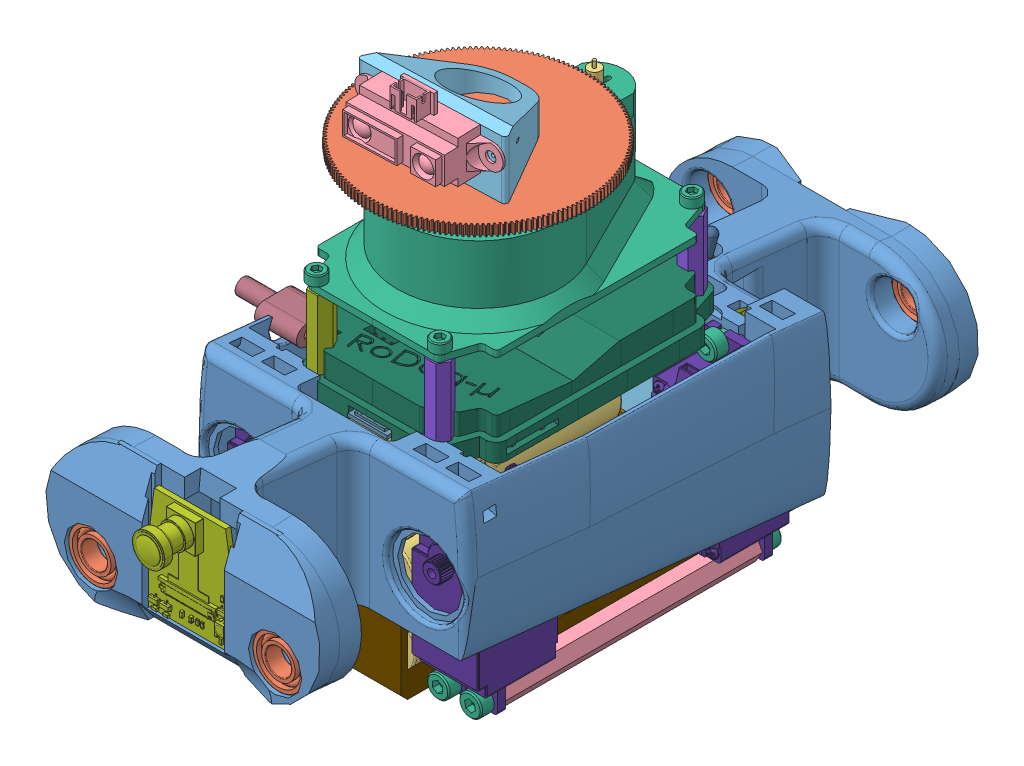
SolidWorks assembly body, configuration Default. Lengths in mm.
Overall size (109.19 147.84 215.45).
83 component instances, 28 part files, 130 mates.
Components (placement in the parent):
- Chasis-1: Chasis [Default] at (0 30 0) x (-1 0 0) z (0 0 1) size (106.67 62.56 205.11)
- radial ball bearing_68_am-1: radial ball bearing_68_am [AFBMA 20.1 - 28-8 - 12,SI,NC,12_68] at (28.5 0 98.3749) x (0 0 -1) z (1 0 0) size (5 16 16)
- radial ball bearing_68_am-2: radial ball bearing_68_am [AFBMA 20.1 - 28-8 - 12,SI,NC,12_68] at (-28.5 0 98.3749) x (0 0 -1) z (1 0 0) size (5 16 16)
- radial ball bearing_68_am-3: radial ball bearing_68_am [AFBMA 20.1 - 28-8 - 12,SI,NC,12_68] at (28.5 0 -98.3749) x (0 0 1) z (-0.94079 -0.338989 0) size (5 16 16)
- radial ball bearing_68_am-4: radial ball bearing_68_am [AFBMA 20.1 - 28-8 - 12,SI,NC,12_68] at (-28.5 0 -98.3749) x (0 0 1) z (-1 0 0) size (5 16 16)
- batteries-1: batteries [Default] at (0 -2.9 15.9266) x (0 -1 0) z (0 0 1) size (60.35 42.06 66)
  - 18650Model-std-11: 18650Model-std [Default] at (-9 -9 -32) x (1 0 0) z (0 0 -1) size (18 18 65)
  - 18650Model-std-12: 18650Model-std [Default] at (9 -9 32) x (-0.155006 -0.987914 0) z (0 0 1) size (18 18 65)
  - 18650Model-std-13: 18650Model-std [Default] at (-9 9 -32) x (0.41216 -0.911111 0) z (0 0 -1) size (18 18 65)
  - 18650Model-std-14: 18650Model-std [Default] at (9 9 32) x (0.93408 -0.357065 0) z (0 0 1) size (18 18 65)
  - 18650Model-std-15: 18650Model-std [Default] at (27 -9 32) x (-0.934528 0.355889 0) z (0 0 1) size (18 18 65)
  - 18650Model-std-16: 18650Model-std [Default] at (27 9 32) x (0.84116 -0.540786 0) z (0 0 1) size (18 18 65)
- 80x4mm standoff-1: 80x4mm standoff [Default] at (33.5 -36.4 -39.9266) x (0.999176 -0.040598 0) z (0 0 1) size (8.08 7 80)
- 80x4mm standoff-2: 80x4mm standoff [Default] at (-33.5 -36.4 -39.9266) x (0.828718 -0.559667 0) z (0 0 1) size (8.08 7 80)
- 1X08-BIG.step-1: 1X08-BIG.step [Default] at (0 -27.0348 -47.5734) x (0 0 -1) z (0 -1 0) size (10 31 29.5)
- socket head cap screw_am-1: socket head cap screw_am [B18.3.1M - 4 x 0.7 x 10 Hex SHCS -- 10NHX] at (-33.5 -36.4 46.5734) x (0 0 -1) z (1 0 0) size (14 7 7)
- socket head cap screw_am-2: socket head cap screw_am [B18.3.1M - 4 x 0.7 x 10 Hex SHCS -- 10NHX] at (-23.5 -36.4 46.5734) x (0 0 -1) z (0.464802 -0.885415 0) size (14 7 7)
- socket head cap screw_am-3: socket head cap screw_am [B18.3.1M - 4 x 0.7 x 10 Hex SHCS -- 10NHX] at (23.5 -36.4 46.5734) x (0 0 -1) z (1 0 0) size (14 7 7)
- socket head cap screw_am-4: socket head cap screw_am [B18.3.1M - 4 x 0.7 x 10 Hex SHCS -- 10NHX] at (33.5 -36.4 46.5734) x (0 0 -1) z (0.972971 0.230929 0) size (14 7 7)
- socket head cap screw_am-5: socket head cap screw_am [B18.3.1M - 4 x 0.7 x 10 Hex SHCS -- 10NHX] at (33.5 -36.4 -46.5734) x (0 0 1) z (-1 0 0) size (14 7 7)
- socket head cap screw_am-6: socket head cap screw_am [B18.3.1M - 4 x 0.7 x 10 Hex SHCS -- 10NHX] at (23.5 -36.4 -46.5734) x (0 0 1) z (-1 0 0) size (14 7 7)
- socket head cap screw_am-7: socket head cap screw_am [B18.3.1M - 4 x 0.7 x 10 Hex SHCS -- 10NHX] at (-33.5 -36.4 -46.5734) x (0 0 1) z (-1 0 0) size (14 7 7)
- socket head cap screw_am-8: socket head cap screw_am [B18.3.1M - 4 x 0.7 x 10 Hex SHCS -- 10NHX] at (-23.5 -36.4 -46.5734) x (0 0 1) z (-1 0 0) size (14 7 7)
- socket head cap screw_am-13: socket head cap screw_am [B18.3.1M - 4 x 0.7 x 10 Hex SHCS -- 10NHX] at (-33.5 13 36.0734) x (0 0 1) z (-0.497518 -0.867454 0) size (14 7 7)
- socket head cap screw_am-14: socket head cap screw_am [B18.3.1M - 4 x 0.7 x 10 Hex SHCS -- 10NHX] at (-23.5 13 36.0734) x (0 0 1) z (-0.937162 -0.348893 0) size (14 7 7)
- socket head cap screw_am-15: socket head cap screw_am [B18.3.1M - 4 x 0.7 x 10 Hex SHCS -- 10NHX] at (23.5 13 -36.0734) x (0 0 -1) z (0.999531 -0.030613 0) size (14 7 7)
- socket head cap screw_am-16: socket head cap screw_am [B18.3.1M - 4 x 0.7 x 10 Hex SHCS -- 10NHX] at (33.5 13 -36.0734) x (0 0 -1) z (0.970522 0.241011 0) size (14 7 7)
- socket head cap screw_am-17: socket head cap screw_am [B18.3.1M - 4 x 0.7 x 10 Hex SHCS -- 10NHX] at (23.5 13 36.0734) x (0 0 1) z (-0.883708 -0.468039 0) size (14 7 7)
- socket head cap screw_am-18: socket head cap screw_am [B18.3.1M - 4 x 0.7 x 10 Hex SHCS -- 10NHX] at (33.5 13 36.0734) x (0 0 1) z (-0.911074 -0.412244 0) size (14 7 7)
- socket head cap screw_am-19: socket head cap screw_am [B18.3.1M - 4 x 0.7 x 10 Hex SHCS -- 10NHX] at (-33.5 13 -36.0734) x (0 0 -1) z (0.998285 -0.058546 0) size (14 7 7)
- socket head cap screw_am-20: socket head cap screw_am [B18.3.1M - 4 x 0.7 x 10 Hex SHCS -- 10NHX] at (-23.5 13 -36.0734) x (0 0 -1) z (0.993249 -0.115998 0) size (14 7 7)
- mobo2_camSLDPRT-1: mobo2_camSLDPRT [Default] at (-51.3967 -126.1208 97.875) x (0 1 0) z (0 0 1) size (33.03 26.96 15.7)
- FUJISOKU ATE 2D.stp-1: FUJISOKU ATE 2D.stp [Default] at (0.3584 5.2835 -67.8989) x (0 0 -1) z (0 1 0) size (9.5 5 23.29)
  - SW7.stp-1: SW7.stp [Default] at (-7.8256 0.3584 -3.9) size (9.5 5 7.8)
  - SW8.stp-1: SW8.stp [Default] at (-7.8256 0.3584 4.4) x (1 0 0) z (0 0 -1) size (9.5 5 10)
  - SW3.stp-1: SW3.stp [Default] at (-7.8256 0.3584 7.4) x (0.978148 0 -0.207912) z (0 -1 0) size (3.5 10.25 3.8)
  - SW10.stp-1: SW10.stp [Default] at (-7.8256 1.6284 -3.4) x (1 0 0) z (0 1 0) size (1 3.81 0.59)
  - SW10.stp-2: SW10.stp [Default] at (-5.2856 1.6284 -3.4) x (1 0 0) z (0 1 0) size (1 3.81 0.59)
  - SW10.stp-3: SW10.stp [Default] at (-10.3656 1.6284 -3.4) x (1 0 0) z (0 1 0) size (1 3.81 0.59)
  - SW10_MIR.stp-1: SW10_MIR.stp [Default] at (-10.3656 -0.9116 -3.4) x (1 0 0) z (0 1 0) size (1 3.81 0.59)
  - SW10_MIR.stp-2: SW10_MIR.stp [Default] at (-5.2856 -0.9116 -3.4) x (1 0 0) z (0 1 0) size (1 3.81 0.59)
  - SW10_MIR.stp-3: SW10_MIR.stp [Default] at (-7.8256 -0.9116 -3.4) x (1 0 0) z (0 1 0) size (1 3.81 0.59)
- USB C mockup-1: USB C mockup [Default] at (-25.8477 21.8173 27.4357) x (0.000257 0 1) z (-1 0 0.000257) size (13 6 30)
- RodogMobo-1: RodogMobo [Default] at (-18.2824 20.1 -37.4091) x (0.000772 0 1) z (0 1 0) size (86.12 60.15 16.5)
- Mobo cover-1: Mobo cover [Default] at (0 19.7 0) x (1 0 0) z (0 1 0) size (60.01 87.25 12.67)
- socket head cap screw_am-21: socket head cap screw_am [B18.3.1M - 3 x 0.5 x 10 Hex SHCS -- 10NHX] at (-18.2187 28.7 40.7111) x (0 -1 0) z (0 0 1) size (13 5.5 5.5) (hidden)
- socket head cap screw_am-22: socket head cap screw_am [B18.3.1M - 3 x 0.5 x 10 Hex SHCS -- 10NHX] at (-18.279 28.7 -37.3889) x (0 -1 0) z (-0.207293 0 -0.978279) size (13 5.5 5.5) (hidden)
- socket head cap screw_am-23: socket head cap screw_am [B18.3.1M - 3 x 0.5 x 10 Hex SHCS -- 10NHX] at (18.221 28.7 -37.4171) x (0 -1 0) z (0 0 1) size (13 5.5 5.5) (hidden)
- socket head cap screw_am-24: socket head cap screw_am [B18.3.1M - 3 x 0.5 x 10 Hex SHCS -- 10NHX] at (18.2813 28.7 40.6829) x (0 -1 0) z (0 0 1) size (13 5.5 5.5) (hidden)
- hex nut style 1_am-2: hex nut style 1_am [B18.2.4.1M - Hex nut, Style 1,  M4 x 0.7 --D-N] at (-33.5 13 50.1734) x (-0.244529 0.969642 0) z (0 0 1) size (7 8.08 3.2)
- hex nut style 1_am-3: hex nut style 1_am [B18.2.4.1M - Hex nut, Style 1,  M4 x 0.7 --D-N] at (-23.5 13 50.1734) x (0.692093 0.721808 0) z (0 0 1) size (7 8.08 3.2)
- hex nut style 1_am-4: hex nut style 1_am [B18.2.4.1M - Hex nut, Style 1,  M4 x 0.7 --D-N] at (33.5 13 46.9734) x (-0.965845 0.259119 0) z (0 0 -1) size (7 8.08 3.2)
- hex nut style 1_am-5: hex nut style 1_am [B18.2.4.1M - Hex nut, Style 1,  M4 x 0.7 --D-N] at (23.5 13 46.9734) x (0.793594 0.608447 0) z (0 0 -1) size (7 8.08 3.2)
- hex nut style 1_am-6: hex nut style 1_am [B18.2.4.1M - Hex nut, Style 1,  M4 x 0.7 --D-N] at (-23.5 13 -50.1734) x (-0.5 0.866025 0) z (0 0 -1) size (7 8.08 3.2)
- hex nut style 1_am-7: hex nut style 1_am [B18.2.4.1M - Hex nut, Style 1,  M4 x 0.7 --D-N] at (23.5 13 -46.9734) x (-1 0 0) z (0 0 1) size (7 8.08 3.2)
- hex nut style 1_am-8: hex nut style 1_am [B18.2.4.1M - Hex nut, Style 1,  M4 x 0.7 --D-N] at (-33.5 13 -46.9734) x (-0.793594 0.608447 0) z (0 0 1) size (7 8.08 3.2)
- hex nut style 1_am-9: hex nut style 1_am [B18.2.4.1M - Hex nut, Style 1,  M4 x 0.7 --D-N] at (33.5 13 -46.9734) x (-0.254777 -0.967 0) z (0 0 1) size (7 8.08 3.2)
- HS-8775MG-1: HS-8775MG [Default] at (-38.5 8 24.0734) x (0 -1 0) z (-1 0 0) size (54.4 29.4 21)
- HS-8775MG-2: HS-8775MG [Default] at (-18.5 8 -24.0734) x (0 -1 0) z (1 0 0) size (54.4 29.4 21)
- HS-8775MG-3: HS-8775MG [Default] at (38.5 8 -24.0734) x (0 -1 0) z (1 0 0) size (54.4 29.4 21)
- HS-8775MG-4: HS-8775MG [Default] at (18.5 8 24.0734) x (0 -1 0) z (-1 0 0) size (54.4 29.4 21)
- Battery mount-1: Battery mount [Default] at (-38.5 8 40.0734) x (0 1 0) z (0 0 -1) size (23.66 55.5 105.15)
- 2D scanner assembly-1: 2D scanner assembly [Default] at (0.0023 52 10.5725) x (0 0 -1) z (1 0 0) size (85.67 58.5 70.17)
  - Slip Ring-1: Slip Ring [Default] at origin size (44 35.4 44)
  - spur gear_am-3: spur gear_am [Metric - Spur gear 0.4M 168T 20PA 3FW ---S168O19H8L12N] at (0 29.5 0) x (0 -1 0) z (0.999472 0 -0.032496) size (8 67.99 67.99)
  - DC Motor-1: DC Motor [Default] at (36 7 0) x (1 0 0) z (0 1 0) size (12.1 10 25)
  - 2Y0A21-1: 2Y0A21 [Default] at (-14.9921 41.0001 0.4874) x (-0.032496 0 -0.999472) z (-0.999472 0 0.032496) size (44.5 19 13.5)
  - Part7^2D scanner assembly-1: Part7^2D scanner assembly [Default] at (0 29.5 0) x (0.999472 0 -0.032496) z (0 1 0) size (28 44.18 18) (virtual)
  - Part8^2D scanner assembly-1: Part8^2D scanner assembly [Default] at (0 19.1 0) x (-1 0 0) z (0 -1 0) size (83.25 58.72 30) (virtual)
  - RodogMobo-1: RodogMobo [Default] at (-30.1305 -16.6 18.2824) x (1 0 -0.000772) z (0 1 0) size (86.12 60.15 16.5) (hidden)
  - socket head cap screw_am-1: socket head cap screw_am [B18.3.1M - 3 x 0.5 x 25 Hex SHCS -- 18NHX] at (0 24.5 -17.4) x (0 -1 0) z (0 0 1) size (28 5.5 5.5)
  - socket head cap screw_am-2: socket head cap screw_am [B18.3.1M - 3 x 0.5 x 25 Hex SHCS -- 18NHX] at (-15.0688 24.5 8.7) x (0 -1 0) z (0 0 1) size (28 5.5 5.5)
  - socket head cap screw_am-3: socket head cap screw_am [B18.3.1M - 3 x 0.5 x 25 Hex SHCS -- 18NHX] at (15.0688 24.5 8.7) x (0 -1 0) z (0 0 1) size (28 5.5 5.5)
- Copy of Part22^body-1: Copy of Part22^body [Default] at (0 25.7 0) x (1 0 0) z (0 1 0) size (6.93 6 21.3) (virtual)
- Part22^body-2: Part22^body [Default] at (-0.6066 25.7 -78.689) x (1 0 -0.000515) z (0 1 0) size (6.93 6 21.3) (virtual)
- Part22^body-3: Part22^body [Default] at (35.8934 25.7 -78.7171) x (1 0 -0.000515) z (0 1 0) size (6.93 6 21.3) (virtual)
- Part22^body-4: Part22^body [Default] at (35.9537 25.7 -0.6172) x (1 0 -0.000515) z (0 1 0) size (6.93 6 21.3) (virtual)
- socket head cap screw_am-25: socket head cap screw_am [B18.3.1M - 3 x 0.5 x 10 Hex SHCS -- 10NHX] at (-18.943 52 41.6116) x (0 -1 0) z (0.000515 0 1) size (13 5.5 5.5)
- socket head cap screw_am-26: socket head cap screw_am [B18.3.1M - 3 x 0.5 x 10 Hex SHCS -- 10NHX] at (18.2813 52 40.6829) x (0 -1 0) z (0.000515 0 1) size (13 5.5 5.5)
- socket head cap screw_am-27: socket head cap screw_am [B18.3.1M - 3 x 0.5 x 10 Hex SHCS -- 10NHX] at (-18.279 52 -37.3889) x (0 -1 0) z (0.000515 0 1) size (13 5.5 5.5)
- socket head cap screw_am-28: socket head cap screw_am [B18.3.1M - 3 x 0.5 x 10 Hex SHCS -- 10NHX] at (18.221 52 -37.4171) x (0 -1 0) z (-0.000515 0 -1) size (13 5.5 5.5)
- power switch-1: power switch [Default] at (0 -40.3958 -30.5734) size (24 22.3 21)
- Part23^body-1: Part23^body [Default] at (0 16.7 0) x (1 0 0) z (0 1 0) (virtual)
Mates (geometry in assembly coordinates):
- Symmetric1: symmetric aligned: plane of Chasis-1 through (-39 -30 42.5734) normal (1 0 0); plane of Chasis-1 through (39 -30 42.5734) normal (-1 0 0)
- Symmetric3: symmetric aligned: plane of Chasis-1 through (15 -30 -52.5734) normal (0 0 1); plane of Chasis-1 through (-15 -30 52.5734) normal (0 0 -1)
- Coincident1: coincident: line of Chasis-1 through (-28.5 0 -95.875) axis (0 0 -1)
- Concentric1: concentric anti-aligned: cylinder of Chasis-1 through (28.5 0 95.8749) axis (0 0 1) radius 8.25; cylinder of radial ball bearing_68_am-1 through (28.5 0 119.0124) axis (0 0 -1) radius 8
- Concentric2: concentric anti-aligned: cylinder of Chasis-1 through (28.5 0 -95.8749) axis (0 0 -1) radius 8.25; cylinder of radial ball bearing_68_am-3 through (28.5 0 -119.0124) axis (0 0 1) radius 8
- Concentric3: concentric anti-aligned: cylinder of Chasis-1 through (-28.5 0 -95.8749) axis (0 0 -1) radius 8.25; cylinder of radial ball bearing_68_am-4 through (-28.5 0 -119.0124) axis (0 0 1) radius 8
- Concentric4: concentric anti-aligned: cylinder of Chasis-1 through (-28.5 0 95.8749) axis (0 0 1) radius 8.25; cylinder of radial ball bearing_68_am-2 through (-28.5 0 119.0124) axis (0 0 -1) radius 8
- Coincident2: coincident anti-aligned: plane of Chasis-1 through (-28.5 0 95.8749) normal (0 0 1); plane of radial ball bearing_68_am-2 through (-28.5 7.8 95.8749) normal (0 0 -1)
- Coincident3: coincident anti-aligned: plane of Chasis-1 through (28.5 0 95.8749) normal (0 0 1); plane of radial ball bearing_68_am-1 through (28.5 7.8 95.8749) normal (0 0 -1)
- Coincident4: coincident anti-aligned: plane of Chasis-1 through (28.5 0 -95.8749) normal (0 0 -1); plane of radial ball bearing_68_am-3 through (25.8559 7.3382 -95.8749) normal (0 0 1)
- Coincident5: coincident anti-aligned: plane of Chasis-1 through (-28.5 0 -95.8749) normal (0 0 -1); plane of radial ball bearing_68_am-4 through (-28.5 7.8 -95.8749) normal (0 0 1)
- Coincident13: coincident aligned: plane of 80x4mm standoff-1 through (33.5 -36.4 -39.9266) normal (0 0 -1); plane of 80x4mm standoff-2 through (-33.5 -36.4 -39.9266) normal (0 0 -1)
- Width3: width anti-aligned: plane of mobo2_camSLDPRT-1 through (13.4799 -42.8697 95.125) normal (1 0 0); plane of mobo2_camSLDPRT-1 through (-13.4799 -6.56 97.875) normal (-1 0 0); plane of Chasis-1 through (13.75 -18.2426 97.875) normal (-1 0 0); plane of Chasis-1 through (-13.75 -18.2426 97.875) normal (1 0 0)
- Coincident35: coincident anti-aligned: plane of Chasis-1 through (12.75 -18.2426 97.875) normal (0 0 1); plane of mobo2_camSLDPRT-1 through (31.7166 15.3847 97.875) normal (0 0 -1)
- Coincident36: coincident: plane of Chasis-1 through (6 -6.56 -101.876) normal (0 1 0); line of mobo2_camSLDPRT-1 through (0.6527 -6.56 97.875) axis (0 0 1)
- Concentric39: concentric anti-aligned: cylinder of Chasis-1 through (0 30.1839 -60.0734) axis (0 -1 0) radius 3.65; cylinder of FUJISOKU ATE 2D.stp-1/SW8.stp-1 through (0 9.6835 -60.0734) axis (0 1 0) radius 2
- Coincident37: coincident anti-aligned: plane of Chasis-1 through (0 9.6835 -67.5734) normal (0 -1 0); plane of FUJISOKU ATE 2D.stp-1/SW8.stp-1 through (0 9.6835 -60.0734) normal (0 1 0)
- Parallel2: parallel aligned: plane of Chasis-1 through (-7 -30 -56.165) normal (-1 0 0); plane of FUJISOKU ATE 2D.stp-1/SW7.stp-1 through (-2.5 1.3835 -64.8234) normal (-1 0 0)
- Tangent7: tangent aligned: cylinder of batteries-1/18650Model-std-16 through (9 -29.9 1047.9266) axis (0 0 1) radius 9; plane of 80x4mm standoff-1 through (31.3388 -39.8151 40.0734) normal (-0.040598 -0.999176 0)
- Parallel6: parallel aligned: plane of Chasis-1 through (-53.3611 16.57 24.2792) normal (0 1 0); plane of USB C mockup-1 through (-45.8486 24.8173 23.9409) normal (0 1 0)
- Coincident46: coincident: line of Chasis-1 through (-39 -27.7348 -52.5734) axis (1 0 0); plane of 1X08-BIG.step-1 through (23 -27.7348 -42.5734) normal (0 -1 0)
- Coincident47: coincident anti-aligned: plane of Chasis-1 through (15 -30 -52.5734) normal (0 0 1); plane of 1X08-BIG.step-1 through (0 -27.0348 -52.5734) normal (0 0 -1)
- Concentric42: concentric anti-aligned: cylinder of Mobo cover-1 through (-18.2187 32.7661 40.7111) axis (0 -1 0) radius 1.5; cylinder of socket head cap screw_am-21 through (-18.2187 60.45 40.7111) axis (0 1 0) radius 2.75
- Coincident54: coincident anti-aligned: plane of Mobo cover-1 through (18.2813 25.7 40.6829) normal (0 1 0); plane of socket head cap screw_am-21 through (-15.4687 25.7 40.7111) normal (0 -1 0)
- Concentric43: concentric anti-aligned: cylinder of Mobo cover-1 through (-18.279 32.7661 -37.3889) axis (0 -1 0) radius 1.5; cylinder of socket head cap screw_am-22 through (-18.279 60.45 -37.3889) axis (0 1 0) radius 2.75
- Coincident55: coincident anti-aligned: plane of Mobo cover-1 through (18.2813 25.7 40.6829) normal (0 1 0); plane of socket head cap screw_am-22 through (-20.9692 25.7 -36.8188) normal (0 -1 0)
- Concentric44: concentric anti-aligned: cylinder of Mobo cover-1 through (18.221 32.7661 -37.4171) axis (0 -1 0) radius 1.5; cylinder of socket head cap screw_am-23 through (18.221 60.45 -37.4171) axis (0 1 0) radius 2.75
- Coincident56: coincident anti-aligned: plane of Mobo cover-1 through (18.2813 25.7 40.6829) normal (0 1 0); plane of socket head cap screw_am-23 through (20.971 25.7 -37.4171) normal (0 -1 0)
- Concentric45: concentric anti-aligned: cylinder of Mobo cover-1 through (18.2813 32.7661 40.6829) axis (0 -1 0) radius 1.5; cylinder of socket head cap screw_am-24 through (18.2813 60.45 40.6829) axis (0 1 0) radius 2.75
- Coincident57: coincident anti-aligned: plane of Mobo cover-1 through (18.2813 25.7 40.6829) normal (0 1 0); plane of socket head cap screw_am-24 through (21.0313 25.7 40.6829) normal (0 -1 0)
- Coincident58: coincident aligned: plane of hex nut style 1_am-2 through (-37.4188 12.0117 50.1734) normal (0 0 1); plane of hex nut style 1_am-3 through (-26.4172 15.7971 50.1734) normal (0 0 1)
- Coincident59: coincident aligned: plane of hex nut style 1_am-4 through (34.5472 16.9034 46.9734) normal (0 0 -1); plane of hex nut style 1_am-5 through (25.959 9.7927 46.9734) normal (0 0 -1)
- Coincident61: coincident aligned: plane of hex nut style 1_am-3 through (-26.4172 15.7971 50.1734) normal (0 0 1); plane of hex nut style 1_am-5 through (25.959 9.7927 50.1734) normal (0 0 1)
- Width19: width aligned: plane of Chasis-1 through (0 30 46.5734) normal (0 0 1); plane of Chasis-1 through (0 30 50.5734) normal (0 0 -1); plane of hex nut style 1_am-5 through (25.959 9.7927 50.1734) normal (0 0 1); plane of hex nut style 1_am-5 through (25.959 9.7927 46.9734) normal (0 0 -1)
- Concentric46: concentric anti-aligned: cylinder of socket head cap screw_am-16 through (33.5 13 -4.3234) axis (0 0 1) radius 3.5; cylinder of hex nut style 1_am-4 through (33.5 13 50.1734) axis (0 0 -1) radius 1.65
- Concentric47: concentric anti-aligned: cylinder of socket head cap screw_am-15 through (23.5 13 -4.3234) axis (0 0 1) radius 2; cylinder of hex nut style 1_am-5 through (23.5 13 50.1734) axis (0 0 -1) radius 1.65
- Concentric48: concentric anti-aligned: cylinder of socket head cap screw_am-13 through (-33.5 13 4.3234) axis (0 0 -1) radius 2; cylinder of hex nut style 1_am-2 through (-33.5 13 46.9734) axis (0 0 1) radius 1.65
- Concentric49: concentric anti-aligned: cylinder of socket head cap screw_am-14 through (-23.5 13 4.3234) axis (0 0 -1) radius 2; cylinder of hex nut style 1_am-3 through (-23.5 13 46.9734) axis (0 0 1) radius 1.65
- Coincident62: coincident aligned: plane of hex nut style 1_am-8 through (-35.959 9.7927 -46.9734) normal (0 0 1); plane of hex nut style 1_am-9 through (37.4081 11.9703 -46.9734) normal (0 0 1)
- Coincident63: coincident aligned: plane of hex nut style 1_am-7 through (23.5 8.9585 -46.9734) normal (0 0 1); plane of hex nut style 1_am-8 through (-35.959 9.7927 -46.9734) normal (0 0 1)
- Coincident64: coincident aligned: plane of hex nut style 1_am-6 through (-20 15.0207 -46.9734) normal (0 0 1); plane of hex nut style 1_am-8 through (-35.959 9.7927 -46.9734) normal (0 0 1)
- Width20: width aligned: plane of Chasis-1 through (0 30 -50.5734) normal (0 0 1); plane of Chasis-1 through (0 30 -46.5734) normal (0 0 -1); plane of hex nut style 1_am-8 through (-35.959 9.7927 -46.9734) normal (0 0 1); plane of hex nut style 1_am-8 through (-35.959 9.7927 -50.1734) normal (0 0 -1)
- Concentric50: concentric anti-aligned: cylinder of socket head cap screw_am-20 through (-23.5 13 -4.3234) axis (0 0 1) radius 2; cylinder of hex nut style 1_am-6 through (-23.5 13 -46.9734) axis (0 0 -1) radius 1.65
- Concentric51: concentric aligned: cylinder of socket head cap screw_am-19 through (-33.5 13 -4.3234) axis (0 0 1) radius 2; cylinder of hex nut style 1_am-8 through (-33.5 13 -50.1734) axis (0 0 1) radius 1.65
- Concentric52: concentric anti-aligned: cylinder of socket head cap screw_am-18 through (33.5 13 4.3234) axis (0 0 -1) radius 2; cylinder of hex nut style 1_am-9 through (33.5 13 -50.1734) axis (0 0 1) radius 1.65
- Concentric53: concentric anti-aligned: cylinder of socket head cap screw_am-17 through (23.5 13 4.3234) axis (0 0 -1) radius 2; cylinder of hex nut style 1_am-7 through (23.5 13 -50.1734) axis (0 0 1) radius 1.65
- Concentric55: concentric aligned: cylinder of Chasis-1 through (-28.5 0 14.2891) axis (0 0 1) radius 10; cylinder of HS-8775MG-1 through (-28.5 0 49.4734) axis (0 0 1) radius 1.2645
- Concentric56: concentric aligned: cylinder of Chasis-1 through (-33.5 13 -68.2302) axis (0 0 1) radius 2; cylinder of HS-8775MG-1 through (-33.5 13 40.0734) axis (0 0 1) radius 2.2
- Coincident67: coincident anti-aligned: plane of Chasis-1 through (-39 -30 42.5734) normal (0 0 -1); plane of HS-8775MG-1 through (-28.5 -11.7 42.5734) normal (0 0 1)
- Concentric57: concentric anti-aligned: cylinder of Chasis-1 through (-23.5 13 -68.2302) axis (0 0 1) radius 2; cylinder of socket head cap screw_am-14 through (-23.5 13 4.3234) axis (0 0 -1) radius 2
- Concentric58: concentric anti-aligned: cylinder of Chasis-1 through (-33.5 13 -68.2302) axis (0 0 1) radius 2; cylinder of socket head cap screw_am-13 through (-33.5 13 4.3234) axis (0 0 -1) radius 2
- Coincident68: coincident aligned: plane of socket head cap screw_am-13 through (-36.5361 14.7413 40.0734) normal (0 0 1); plane of socket head cap screw_am-14 through (-24.7211 16.2801 40.0734) normal (0 0 1)
- Coincident69: coincident anti-aligned: plane of socket head cap screw_am-14 through (-24.7211 16.2801 40.0734) normal (0 0 1); plane of HS-8775MG-1 through (-28.5 -11.7 40.0734) normal (0 0 -1)
- Concentric59: concentric aligned: cylinder of socket head cap screw_am-1 through (-33.5 -36.4 78.3234) axis (0 0 1) radius 2; cylinder of HS-8775MG-1 through (-33.5 -36.4 40.0734) axis (0 0 1) radius 2.2
- Concentric60: concentric aligned: cylinder of socket head cap screw_am-2 through (-23.5 -36.4 78.3234) axis (0 0 1) radius 2; cylinder of HS-8775MG-1 through (-23.5 -36.4 40.0734) axis (0 0 1) radius 2.2
- Coincident70: coincident aligned: plane of socket head cap screw_am-1 through (-33.5 -32.9 42.5734) normal (0 0 -1); plane of socket head cap screw_am-2 through (-20.401 -34.7732 42.5734) normal (0 0 -1)
- Coincident71: coincident anti-aligned: plane of socket head cap screw_am-2 through (-20.401 -34.7732 42.5734) normal (0 0 -1); plane of HS-8775MG-1 through (-28.5 -11.7 42.5734) normal (0 0 1)
- Coincident73: coincident aligned: plane of batteries-1 through (0 -2.9 15.9266) normal (1 0 0)
- Tangent10: tangent aligned: cylinder of batteries-1/18650Model-std-15 through (-9 -29.9 1047.9266) axis (0 0 1) radius 9; plane of HS-8775MG-1 through (-22.25 -38.9 40.0734) normal (0 -1 0)
- Concentric61: concentric anti-aligned: cylinder of Chasis-1 through (-23.5 13 -68.2302) axis (0 0 1) radius 2; cylinder of HS-8775MG-2 through (-23.5 13 -40.0734) axis (0 0 -1) radius 2.2
- Concentric62: concentric anti-aligned: cylinder of Chasis-1 through (-33.5 13 -68.2302) axis (0 0 1) radius 2; cylinder of HS-8775MG-2 through (-33.5 13 -40.0734) axis (0 0 -1) radius 2.2
- Coincident74: coincident anti-aligned: plane of Chasis-1 through (-39 -30 -42.5734) normal (0 0 1); plane of HS-8775MG-2 through (-28.5 -11.7 -42.5734) normal (0 0 -1)
- Coincident75: coincident aligned: plane of socket head cap screw_am-19 through (-33.2951 16.494 -40.0734) normal (0 0 -1); plane of socket head cap screw_am-20 through (-23.094 16.4764 -40.0734) normal (0 0 -1)
- Coincident76: coincident anti-aligned: plane of socket head cap screw_am-19 through (-33.2951 16.494 -40.0734) normal (0 0 -1); plane of HS-8775MG-2 through (-28.5 -11.7 -40.0734) normal (0 0 1)
- Concentric63: concentric anti-aligned: cylinder of socket head cap screw_am-20 through (-23.5 13 -4.3234) axis (0 0 1) radius 2; cylinder of HS-8775MG-2 through (-23.5 13 -40.0734) axis (0 0 -1) radius 2.2
- Concentric64: concentric anti-aligned: cylinder of socket head cap screw_am-19 through (-33.5 13 -4.3234) axis (0 0 1) radius 2; cylinder of HS-8775MG-2 through (-33.5 13 -40.0734) axis (0 0 -1) radius 2.2
- Concentric65: concentric aligned: cylinder of Chasis-1 through (23.5 13 -68.2302) axis (0 0 1) radius 2; cylinder of HS-8775MG-4 through (23.5 13 40.0734) axis (0 0 1) radius 2.2
- Concentric66: concentric aligned: cylinder of Chasis-1 through (33.5 13 -68.2302) axis (0 0 1) radius 2; cylinder of HS-8775MG-4 through (33.5 13 40.0734) axis (0 0 1) radius 2.2
- Coincident77: coincident anti-aligned: plane of Chasis-1 through (39 -30 42.5734) normal (0 0 -1); plane of HS-8775MG-4 through (28.5 -11.7 42.5734) normal (0 0 1)
- Concentric67: concentric anti-aligned: cylinder of Chasis-1 through (23.5 13 -68.2302) axis (0 0 1) radius 2; cylinder of socket head cap screw_am-17 through (23.5 13 4.3234) axis (0 0 -1) radius 2
- Concentric68: concentric anti-aligned: cylinder of Chasis-1 through (33.5 13 -68.2302) axis (0 0 1) radius 2; cylinder of socket head cap screw_am-18 through (33.5 13 4.3234) axis (0 0 -1) radius 2
- Coincident78: coincident aligned: plane of socket head cap screw_am-17 through (21.8619 16.093 40.0734) normal (0 0 1); plane of socket head cap screw_am-18 through (32.0571 16.1888 40.0734) normal (0 0 1)
- Coincident79: coincident anti-aligned: plane of socket head cap screw_am-18 through (32.0571 16.1888 40.0734) normal (0 0 1); plane of HS-8775MG-4 through (28.5 -11.7 40.0734) normal (0 0 -1)
- Concentric69: concentric anti-aligned: cylinder of Chasis-1 through (33.5 13 -68.2302) axis (0 0 1) radius 2; cylinder of HS-8775MG-3 through (33.5 13 -40.0734) axis (0 0 -1) radius 2.2
- Concentric70: concentric anti-aligned: cylinder of Chasis-1 through (23.5 13 -68.2302) axis (0 0 1) radius 2; cylinder of HS-8775MG-3 through (23.5 13 -40.0734) axis (0 0 -1) radius 2.2
- Coincident80: coincident anti-aligned: plane of Chasis-1 through (39 -30 -42.5734) normal (0 0 1); plane of HS-8775MG-3 through (28.5 -11.7 -42.5734) normal (0 0 -1)
- Concentric71: concentric aligned: cylinder of Chasis-1 through (23.5 13 -68.2302) axis (0 0 1) radius 2; cylinder of socket head cap screw_am-15 through (23.5 13 -4.3234) axis (0 0 1) radius 2
- Concentric72: concentric aligned: cylinder of Chasis-1 through (33.5 13 -68.2302) axis (0 0 1) radius 2; cylinder of socket head cap screw_am-16 through (33.5 13 -4.3234) axis (0 0 1) radius 2
- Coincident81: coincident aligned: plane of socket head cap screw_am-15 through (23.6071 16.4984 -40.0734) normal (0 0 -1); plane of socket head cap screw_am-16 through (32.6565 16.3968 -40.0734) normal (0 0 -1)
- Coincident82: coincident anti-aligned: plane of socket head cap screw_am-16 through (32.6565 16.3968 -40.0734) normal (0 0 -1); plane of HS-8775MG-3 through (28.5 -11.7 -40.0734) normal (0 0 1)
- Concentric73: concentric aligned: cylinder of 80x4mm standoff-2 through (-33.5 -36.4 33.9734) axis (0 0 1) radius 1.75; cylinder of socket head cap screw_am-1 through (-33.5 -36.4 78.3234) axis (0 0 1) radius 2
- Coincident83: coincident anti-aligned: plane of 80x4mm standoff-2 through (-33.5 -36.4 40.0734) normal (0 0 1); plane of HS-8775MG-1 through (-28.5 -11.7 40.0734) normal (0 0 -1)
- Concentric74: concentric aligned: cylinder of 80x4mm standoff-1 through (33.5 -36.4 33.9734) axis (0 0 1) radius 1.75; cylinder of socket head cap screw_am-4 through (33.5 -36.4 78.3234) axis (0 0 1) radius 2
- Concentric75: concentric aligned: cylinder of socket head cap screw_am-4 through (33.5 -36.4 78.3234) axis (0 0 1) radius 3.5; cylinder of HS-8775MG-4 through (33.5 -36.4 40.0734) axis (0 0 1) radius 2.2
- Coincident84: coincident anti-aligned: plane of socket head cap screw_am-4 through (32.6917 -32.9946 42.5734) normal (0 0 -1); plane of HS-8775MG-4 through (28.5 -11.7 42.5734) normal (0 0 1)
- Concentric76: concentric aligned: cylinder of socket head cap screw_am-3 through (23.5 -36.4 78.3234) axis (0 0 1) radius 2; cylinder of HS-8775MG-4 through (23.5 -36.4 40.0734) axis (0 0 1) radius 2.2
- Coincident85: coincident aligned: plane of socket head cap screw_am-3 through (23.5 -36.4 46.5734) normal (0 0 1); plane of socket head cap screw_am-4 through (33.5 -36.4 46.5734) normal (0 0 1)
- Coincident86: coincident aligned: plane of socket head cap screw_am-5 through (33.5 -32.9 -42.5734) normal (0 0 1); plane of socket head cap screw_am-6 through (23.5 -32.9 -42.5734) normal (0 0 1)
- Coincident87: coincident anti-aligned: plane of socket head cap screw_am-6 through (23.5 -32.9 -42.5734) normal (0 0 1); plane of HS-8775MG-3 through (28.5 -11.7 -42.5734) normal (0 0 -1)
- Concentric77: concentric aligned: cylinder of socket head cap screw_am-5 through (33.5 -36.4 -78.3234) axis (0 0 -1) radius 2; cylinder of HS-8775MG-3 through (33.5 -36.4 -40.0734) axis (0 0 -1) radius 2.2
- Concentric78: concentric aligned: cylinder of socket head cap screw_am-6 through (23.5 -36.4 -78.3234) axis (0 0 -1) radius 2; cylinder of HS-8775MG-3 through (23.5 -36.4 -40.0734) axis (0 0 -1) radius 2.2
- Coincident88: coincident aligned: plane of socket head cap screw_am-7 through (-33.5 -32.9 -42.5734) normal (0 0 1); plane of socket head cap screw_am-8 through (-23.5 -32.9 -42.5734) normal (0 0 1)
- Coincident89: coincident anti-aligned: plane of socket head cap screw_am-8 through (-23.5 -32.9 -42.5734) normal (0 0 1); plane of HS-8775MG-2 through (-28.5 -11.7 -42.5734) normal (0 0 -1)
- Concentric79: concentric aligned: cylinder of socket head cap screw_am-8 through (-23.5 -36.4 -78.3234) axis (0 0 -1) radius 2; cylinder of HS-8775MG-2 through (-23.5 -36.4 -40.0734) axis (0 0 -1) radius 2.2
- Concentric80: concentric aligned: cylinder of socket head cap screw_am-7 through (-33.5 -36.4 -78.3234) axis (0 0 -1) radius 2; cylinder of HS-8775MG-2 through (-33.5 -36.4 -40.0734) axis (0 0 -1) radius 2.2
- InPlace3: in place: plane of ? through (-28.5 -11.7 30.3127) normal (0 0 -1); plane of ? through (0 0 30.3127) normal (0 0 -1); moOrthogonalPlaneRef_w of ? through (-28.5 -11.7 30.3127) normal (0 0 -1); plane of ? through (0 0 30.3127) normal (0 1 0); plane of ? through (-28.5 -11.7 30.3127) normal (0 0 -1); plane of ? through (0 0 30.3127) normal (-1 0 0); plane of HS-8775MG-1 through (-28.5 -11.7 40.0734) normal (0 0 -1); unknown of Battery mount-1
- Coincident90: coincident aligned: plane of HS-8775MG-1; plane of Battery mount-1
- Coincident91: coincident aligned: plane of HS-8775MG-1 through (-38.5 8 40.0734) normal (1 0 0); plane of Battery mount-1 through (-38.5 8 40.0734) normal (1 0 0)
- Coincident92: coincident anti-aligned: plane of HS-8775MG-1 through (-38.5 8 40.0734) normal (0 -1 0); plane of Battery mount-1 through (-38.5 8 40.0734) normal (0 1 0)
- Concentric81: concentric anti-aligned: cylinder of socket head cap screw_am-24 through (18.2813 60.45 40.6829) axis (0 1 0) radius 2.75; cylinder of 2D scanner assembly-1/Part8^2D scanner assembly-1 through (18.2813 49 40.6829) axis (0 -1 0) radius 1.55
- Concentric82: concentric anti-aligned: cylinder of socket head cap screw_am-22 through (-18.279 60.45 -37.3889) axis (0 1 0) radius 1.5; cylinder of 2D scanner assembly-1/Part8^2D scanner assembly-1 through (-18.279 49 -37.3889) axis (0 -1 0) radius 1.55
- Distance2: distance = 25.3 mm anti-aligned: plane of RodogMobo-1 through (15.8169 21.7 3.174) normal (0 1 0); plane of 2D scanner assembly-1/Part8^2D scanner assembly-1 through (0.0023 47 10.5725) normal (0 -1 0)
- InPlace4: in place: plane of ? through (18.2574 24.6 40.3173) normal (0 1 0); plane of ? through (0 24.6 0) normal (0 1 0); plane of ? through (18.2574 24.6 40.3173) normal (0 1 0); plane of ? through (0 24.6 0) normal (0 0 -1); plane of ? through (18.2574 24.6 40.3173) normal (0 1 0); plane of ? through (0 24.6 0) normal (1 0 0); plane of Mobo cover-1 through (18.2813 25.7 40.6829) normal (0 1 0); unknown of Copy of Part22^body-1
- Coincident90: coincident aligned: plane of Mobo cover-1; plane of Copy of Part22^body-1
- Coincident91: coincident aligned: plane of Mobo cover-1 through (0 25.7 0) normal (0 0 -1); plane of Part22^body-1 through (0 25.7 0) normal (0 0 -1)
- Coincident92: coincident anti-aligned: plane of Mobo cover-1 through (0 25.7 0) normal (-1 0 0); plane of Part22^body-1 through (0 25.7 0) normal (1 0 0)
- Coincident93: coincident aligned: plane of Part22^body-2 through (-0.058 47 -67.5274) normal (0 1 0); plane of Part22^body-3 through (36.442 47 -67.5556) normal (0 1 0)
- Coincident94: coincident aligned: plane of Part22^body-3 through (36.442 47 -67.5556) normal (0 1 0); plane of Part22^body-4 through (36.5023 47 10.5444) normal (0 1 0)
- Coincident95: coincident anti-aligned: plane of 2D scanner assembly-1/Part8^2D scanner assembly-1 through (0.0023 47 10.5725) normal (0 -1 0); plane of Part22^body-3 through (36.442 47 -67.5556) normal (0 1 0)
- Concentric83: concentric aligned: cylinder of 2D scanner assembly-1/Part8^2D scanner assembly-1 through (18.2813 49 40.6829) axis (0 -1 0) radius 1.55; cylinder of Part22^body-4 through (18.2813 56.1652 40.6829) axis (0 -1 0) radius 1.5
- Concentric84: concentric aligned: cylinder of 2D scanner assembly-1/Part8^2D scanner assembly-1 through (-18.279 49 -37.3889) axis (0 -1 0) radius 1.55; cylinder of Part22^body-2 through (-18.279 56.1652 -37.3889) axis (0 -1 0) radius 1.5
- Concentric85: concentric aligned: cylinder of 2D scanner assembly-1/Part8^2D scanner assembly-1 through (18.221 49 -37.4171) axis (0 -1 0) radius 1.55; cylinder of Part22^body-3 through (18.221 56.1652 -37.4171) axis (0 -1 0) radius 1.5
- Concentric86: concentric anti-aligned: cylinder of 2D scanner assembly-1/Part8^2D scanner assembly-1 through (-18.943 49 41.6116) axis (0 -1 0) radius 1.6272; cylinder of socket head cap screw_am-25 through (-18.943 83.75 41.6116) axis (0 1 0) radius 2.75
- Coincident96: coincident anti-aligned: plane of 2D scanner assembly-1/Part8^2D scanner assembly-1 through (0.0023 49 10.5725) normal (0 1 0); plane of socket head cap screw_am-25 through (-16.193 49 41.6102) normal (0 -1 0)
- Concentric87: concentric anti-aligned: cylinder of 2D scanner assembly-1/Part8^2D scanner assembly-1 through (18.2813 49 40.6829) axis (0 -1 0) radius 1.55; cylinder of socket head cap screw_am-26 through (18.2813 83.75 40.6829) axis (0 1 0) radius 2.75
- Coincident97: coincident anti-aligned: plane of 2D scanner assembly-1/Part8^2D scanner assembly-1 through (0.0023 49 10.5725) normal (0 1 0); plane of socket head cap screw_am-26 through (21.0313 49 40.6815) normal (0 -1 0)
- Concentric88: concentric anti-aligned: cylinder of 2D scanner assembly-1/Part8^2D scanner assembly-1 through (-18.279 49 -37.3889) axis (0 -1 0) radius 1.55; cylinder of socket head cap screw_am-27 through (-18.279 83.75 -37.3889) axis (0 1 0) radius 2.75
- Coincident98: coincident anti-aligned: plane of 2D scanner assembly-1/Part8^2D scanner assembly-1 through (0.0023 49 10.5725) normal (0 1 0); plane of socket head cap screw_am-27 through (-15.529 49 -37.3903) normal (0 -1 0)
- Concentric891: concentric anti-aligned: cylinder of 2D scanner assembly-1/Part8^2D scanner assembly-1 through (18.221 49 -37.4171) axis (0 -1 0) radius 1.55; cylinder of socket head cap screw_am-28 through (18.221 83.75 -37.4171) axis (0 1 0) radius 2.75
- Coincident991: coincident anti-aligned: plane of 2D scanner assembly-1/Part8^2D scanner assembly-1 through (0.0023 49 10.5725) normal (0 1 0); plane of socket head cap screw_am-28 through (15.471 49 -37.4157) normal (0 -1 0)
- Width21: width aligned: plane of Chasis-1 through (-39 -30 42.5734) normal (1 0 0); plane of RodogMobo-1 through (39 -30 42.5734) normal (-1 0 0); plane of Chasis-1 through (-27.9704 20.1 31.8884) normal (-1 0 0.000329); plane of RodogMobo-1 through (27.9828 17.85 -5.7329) normal (1 0 0.000329)
- Width22: width aligned: plane of 1X08-BIG.step-1 through (-15.5 -27.0348 -52.5734) normal (-1 0 0); plane of 1X08-BIG.step-1 through (15.5 -9.0348 -52.5734) normal (1 0 0); plane of power switch-1 through (-12 -38.3958 -20.0734) normal (-1 0 0); plane of power switch-1 through (12 -38.3958 -20.0734) normal (1 0 0)
- Distance4: distance = 4 mm anti-aligned: plane of batteries-1/18650Model-std-16 through (11.5866 -31.5629 -17.0734) normal (0 0 -1); plane of power switch-1 through (-11 -24.8958 -21.0734) normal (0 0 1)
- Coincident993: coincident aligned: plane of 1X08-BIG.step-1 through (-15.5 -27.0348 -52.5734) normal (-1 0 0); plane of Battery mount-1 through (-15.5 -73.8211 -42.5734) normal (-1 0 0)
- Coincident995: coincident anti-aligned: plane of Battery mount-1 through (-15.5 -73.8211 -40.0734) normal (0 0 1); plane of power switch-1 through (-11 -24.8958 -40.0734) normal (0 0 -1)
- Coincident996: coincident anti-aligned: plane of Battery mount-1 through (-38.5 -38.3958 40.0734) normal (0 -1 0); plane of power switch-1 through (0 -38.3958 -30.5734) normal (0 1 0)
- InPlace5: in place: plane of Chasis-1 through (0 16.7 0) normal (0 1 0); plane of Part23^body-1 through (0 16.7 0) normal (0 1 0); plane of Chasis-1 through (0 16.7 0) normal (0 1 0); plane of Part23^body-1 through (0 16.7 0) normal (0 0 -1); plane of Chasis-1 through (0 16.7 0) normal (0 1 0); plane of Part23^body-1 through (0 16.7 0) normal (1 0 0); plane of Chasis-1 through (0 16.7 0) normal (0 1 0); unknown of Part23^body-1
- Coincident997: coincident aligned: plane of Chasis-1; plane of Part23^body-1
- Coincident998: coincident aligned: plane of Chasis-1 through (0 16.7 0) normal (0 0 -1); plane of Part23^body-1 through (0 16.7 0) normal (0 0 -1)
- Coincident999: coincident anti-aligned: plane of Chasis-1 through (0 16.7 0) normal (-1 0 0); plane of Part23^body-1 through (0 16.7 0) normal (1 0 0)
